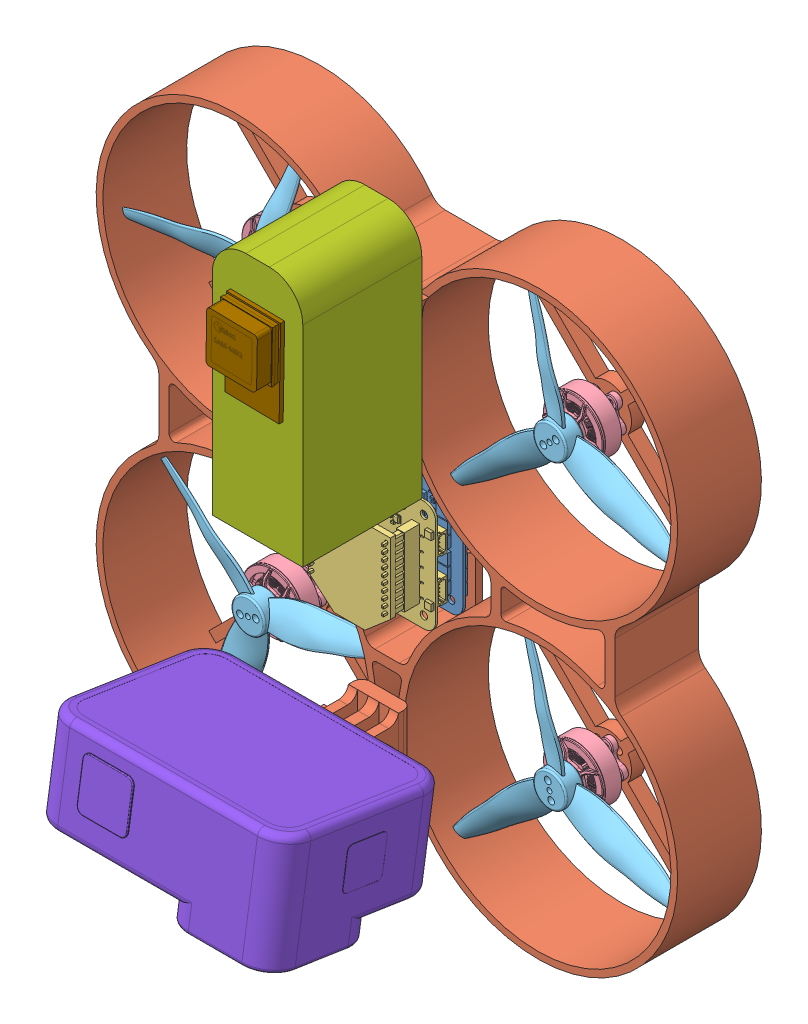
SolidWorks assembly Quad_assem, configuration Default. Lengths in mm.
Overall size (173.5 177.85 96.91).
15 component instances, 9 part files, 29 mates.
Components (placement in the parent):
- 4in1_ESC-1: 4in1_ESC [Default] at (-19 -71.0915 69.7585) x (-1 0 0) z (0 0 1) size (33 33 7.6)
- Quad-1: Quad [Default] at (-19 -71.0915 50.9225) x (-1 0 0) z (0 1 0) size (173.5 44 173.5)
- FlightController.step-1: FlightController.step [Default] at (-19 -71.0915 77.8822) x (-1 0 0) z (0 0 1) size (33 33 15.78)
- 1404 motor.step-5: 1404 motor.step [Default] at (26 -116.0915 54.9225) x (-0.288132 -0.957591 0) z (0 0 1) size (17.9 17.9 14.53)
- Prop-1: Prop [Default] at (26 -116.0915 69.6725) x (-0.210639 0.977564 0) z (0.977564 0.210639 0) size (58.53 5.95 67.58)
- Prop-2: Prop [Default] at (-64 -116.0915 69.6725) x (0.970142 0.242537 0) z (0.242537 -0.970142 0) size (58.53 5.95 67.58)
- 1404 motor.step-6: 1404 motor.step [Default] at (-64 -116.0915 54.9225) x (0.326411 0.945228 0) z (0 0 1) size (17.9 17.9 14.53)
- Prop-3: Prop [Default] at (26 -26.0915 69.6725) x (-0.761093 -0.648643 0) z (-0.648643 0.761093 0) size (58.53 5.95 67.58)
- 1404 motor.step-7: 1404 motor.step [Default] at (26 -26.0915 54.9225) x (0.821885 -0.569654 0) z (0 0 1) size (17.9 17.9 14.53)
- Prop-4: Prop [Default] at (-64 -26.0915 69.6725) x (-0.990537 -0.137246 0) z (-0.137246 0.990537 0) size (58.53 5.95 67.58)
- 1404 motor.step-8: 1404 motor.step [Default] at (-64 -26.0915 54.9225) x (0.979794 -0.200008 0) z (0 0 1) size (17.9 17.9 14.53)
- ToF-1: ToF [Default] at (-19 -71.0915 64.9225) x (1 0 0) z (0 1 0) size (34.5 13.5 18.5)
- Battery-1: Battery [Default] at (-5 -16.2877 97.2725) x (0 -1 0) z (-1 0 0) size (72.6 35.5 27)
- GoPro Hero 9-1: GoPro Hero 9 [Default] at (-54.98 -99.2984 142.2602) x (1 0 0) z (0 -0.151026 -0.98853) size (72.1 33.6 50.5)
- GPS_sam-m8q-2: GPS_sam-m8q [Default] at (-26.1885 8.2042 116.2725) x (0.999848 -0.017452 0) z (-0.017452 -0.999848 0) size (16.15 7.55 26.25)
Mates (geometry in assembly coordinates):
- Concentric3: concentric aligned: circle of 4in1_ESC-1; circle of FlightController.step-1
- Concentric4: concentric aligned: circle of 4in1_ESC-1; circle of FlightController.step-1
- Distance3: distance = 7.5 mm anti-aligned: plane of 4in1_ESC-1 through (-2.5 -58.0915 69.7585) normal (0 0 1); plane of FlightController.step-1 through (-2.5 -58.0915 77.2585) normal (0 0 -1)
- Concentric5: concentric aligned: circle of 1404 motor.step-5; circle of Prop-1
- Concentric6: concentric aligned: circle of Prop-2; circle of 1404 motor.step-6
- Concentric7: concentric aligned: circle of Prop-3; circle of 1404 motor.step-7
- Concentric8: concentric aligned: circle of Prop-4; circle of 1404 motor.step-8
- Coincident11: coincident aligned: plane of Quad-1 through (0 -71.0915 79.9225) normal (1 0 0)
- Coincident17: coincident anti-aligned: plane of Prop-4 through (-64 -26.0915 66.9225) normal (0 0 -1); plane of 1404 motor.step-8 through (-64 -26.0915 66.9225) normal (0 0 1)
- Coincident18: coincident anti-aligned: plane of Prop-3 through (26 -26.0915 66.9225) normal (0 0 -1); plane of 1404 motor.step-7 through (26 -26.0915 66.9225) normal (0 0 1)
- Coincident19: coincident anti-aligned: plane of Prop-2 through (-64 -116.0915 66.9225) normal (0 0 -1); plane of 1404 motor.step-6 through (-64 -116.0915 66.9225) normal (0 0 1)
- Coincident20: coincident anti-aligned: plane of 1404 motor.step-5 through (26 -116.0915 66.9225) normal (0 0 1); plane of Prop-1 through (26 -116.0915 66.9225) normal (0 0 -1)
- Concentric9: concentric anti-aligned: circle of Quad-1; circle of 1404 motor.step-7
- Concentric10: concentric anti-aligned: circle of Quad-1; circle of 1404 motor.step-5
- Concentric11: concentric anti-aligned: circle of Quad-1; circle of 1404 motor.step-6
- Concentric12: concentric anti-aligned: circle of Quad-1; circle of 1404 motor.step-8
- Coincident28: coincident anti-aligned: plane of Quad-1 through (-19 -71.0915 54.9225) normal (0 0 1); plane of 1404 motor.step-6 through (-64 -116.0915 54.9225) normal (0 0 -1)
- Coincident29: coincident anti-aligned: plane of Quad-1 through (-19 -71.0915 54.9225) normal (0 0 1); plane of 1404 motor.step-8 through (-64 -26.0915 54.9225) normal (0 0 -1)
- Coincident30: coincident anti-aligned: plane of Quad-1 through (26 -116.0915 54.9225) normal (0 0 1); plane of 1404 motor.step-5 through (26 -116.0915 54.9225) normal (0 0 -1)
- Coincident31: coincident anti-aligned: plane of Quad-1 through (-19 -71.0915 54.9225) normal (0 0 1); plane of 1404 motor.step-7 through (26 -26.0915 54.9225) normal (0 0 -1)
- Coincident32: coincident anti-aligned: plane of Quad-1 through (-4.5 -56.5915 64.9225) normal (0 0 -1); plane of ToF-1 through (-8.3 -64.3415 64.9225) normal (0 0 1)
- Concentric13: concentric anti-aligned: circle of Quad-1; circle of ToF-1
- Concentric14: concentric anti-aligned: circle of Quad-1; circle of ToF-1
- Distance4: distance = 2 mm anti-aligned: plane of Quad-1 through (-4.5 -56.5915 66.9225) normal (0 0 1); plane of 4in1_ESC-1 through (-2.5 -58.0915 68.9225) normal (0 0 -1)
- Distance6: distance = 5 mm aligned: plane of Battery-1 through (-5 -16.2877 97.2725) normal (1 0 0)
- Coincident33: coincident anti-aligned: plane of Quad-1 through (-19 -71.0915 79.5225) normal (0 0 1); plane of Battery-1 through (-32 20.0123 79.5225) normal (0 0 -1)
- Distance7: distance = 55 mm anti-aligned: plane of GoPro Hero 9-1 through (-55 -99.2984 142.2602) normal (-1 0 0)
- Tangent1: tangent anti-aligned: plane of GoPro Hero 9-1 through (9.02 -134.232 97.0171) normal (0 -0.151026 -0.98853); cylinder of Quad-1 through (-19 -121.0915 87.4225) axis (-1 0 0) radius 7.5
- Coincident36: coincident anti-aligned: plane of Battery-1 through (-32 20.0123 115.0225) normal (0 0 1); plane of GPS_sam-m8q-2 through (-12.8086 -32.0345 115.0225) normal (0 0 -1)
